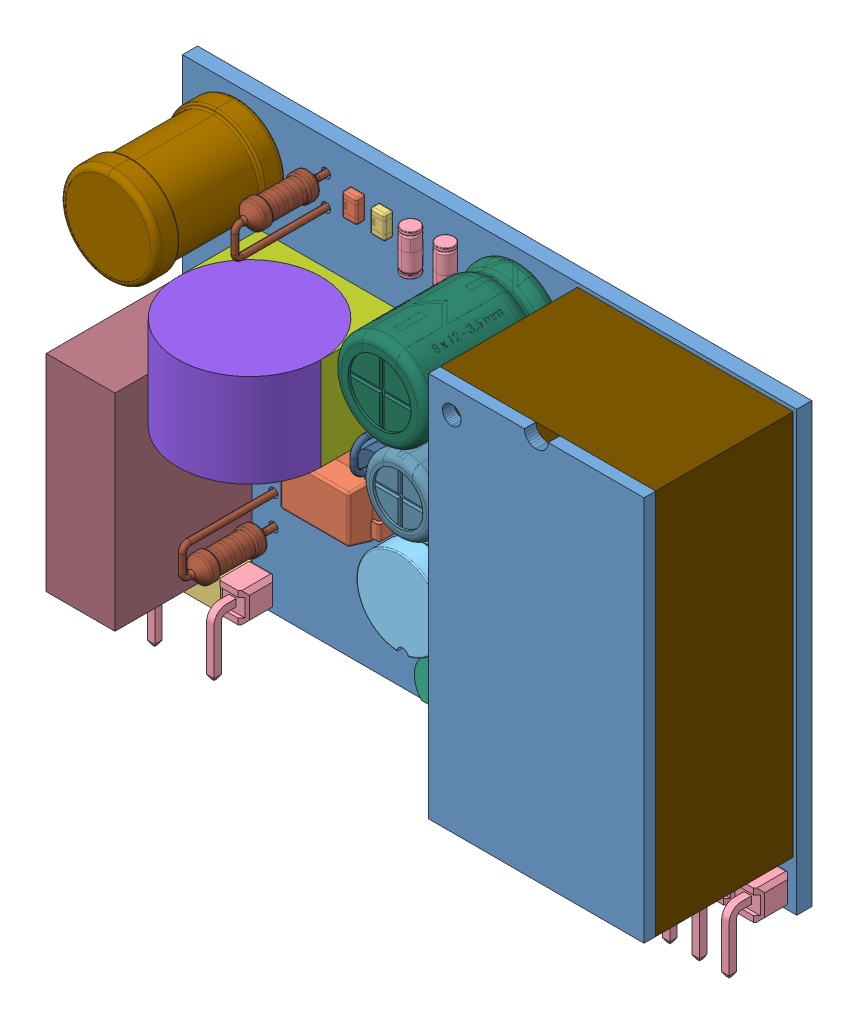
SolidWorks assembly KQ-130F, configuration Default. Lengths in mm.
Overall size (52.7 40.92 18.15).
108 component instances, 25 part files, 0 mates.
Components (placement in the parent):
- KQ-130F.step-1: KQ-130F.step [Default] at origin size (52.7 40.92 18.15)
  - Board.step-1: Board.step [Default] at origin size (52.7 37.6 1.29)
    - Open CASCADE STEP translator 6.8 4.1.1.step-1: Open CASCADE STEP translator 6.8 4.1.1.step [Default] at (0 0 -1.2914) size (52.7 37.6 1.29)
  - Designator39.step-1: Designator39.step [Default] at origin size (1.25 2 0.78)
    - User_Library-0805_SMD_Resistor.step-1: User_Library-0805_SMD_Resistor.step [Default] at (77.385 48.11 0) x (0 1 0) z (1 0 0) size (2 0.78 1.25)
  - Designator38.step-1: Designator38.step [Default] at origin size (1.25 2 0.78)
    - SW3dPS-0805_SMD_Capacitor.step-1: SW3dPS-0805_SMD_Capacitor.step [Default] at (77.345 42.3 0) x (0 1 0) z (1 0 0) size (2 0.78 1.25)
  - Designator37.step-1: Designator37.step [Default] at origin size (1.25 2 0.78)
    - User_Library-0805_SMD_Resistor.step-1: User_Library-0805_SMD_Resistor.step [Default] at (67.215 44.89 0) x (0 -1 0) z (-1 0 0) size (2 0.78 1.25)
  - Designator36.step-1: Designator36.step [Default] at origin size (1.51 3.5 1.51)
    - User_Library-Diode_MELF.step-1: User_Library-Diode_MELF.step [Default] at (63.8201 43.3999 0.75) x (0 1 0) z (0 0 1) size (3.5 1.51 1.51)
  - Designator35.step-1: Designator35.step [Default] at origin size (3.5 1.51 1.51)
    - User_Library-Diode_MELF.step-1: User_Library-Diode_MELF.step [Default] at (54.6999 53.3999 0.75) x (1 0 0) z (0 0 1) size (3.5 1.51 1.51)
  - Designator34.step-1: Designator34.step [Default] at origin size (1.51 3.5 1.51)
    - User_Library-Diode_MELF.step-1: User_Library-Diode_MELF.step [Default] at (65.2999 68.7001 0.75) x (0 -1 0) z (0 0 1) size (3.5 1.51 1.51)
  - Designator33.step-1: Designator33.step [Default] at origin size (1.25 2 0.78)
    - SW3dPS-0805_SMD_Capacitor.step-1: SW3dPS-0805_SMD_Capacitor.step [Default] at (62.485 69.1 0) x (0 1 0) z (1 0 0) size (2 0.78 1.25)
  - Designator32.step-1: Designator32.step [Default] at origin size (1.51 3.5 1.51)
    - User_Library-Diode_MELF.step-1: User_Library-Diode_MELF.step [Default] at (68.3001 68.9999 0.75) x (0 1 0) z (0 0 1) size (3.5 1.51 1.51)
  - Designator31.step-1: Designator31.step [Default] at origin size (1.25 2 0.78)
    - User_Library-0805_SMD_Resistor.step-1: User_Library-0805_SMD_Resistor.step [Default] at (60.085 69.11 0) x (0 1 0) z (1 0 0) size (2 0.78 1.25)
  - Designator30.step-1: Designator30.step [Default] at origin size (1.6 3.2 1)
    - User_Library-1206_SMD_Capacitor.step-1: User_Library-1206_SMD_Capacitor.step [Default] at (69.9999 60 0) x (0 1 0) z (1 0 0) size (3.2 1 1.6)
  - Designator17.step-1: Designator17.step [Default] at origin size (5.58 3.97 7.7)
    - TO-92-1.step-1: TO-92-1.step [Default] at (72.6601 41.8789 0.7086) x (1 0 0) z (0 0 1) size (5.58 3.97 7.7)
  - Designator16.step-1: Designator16.step [Default] at origin size (12.3 8 13.15)
    - 5896934704.step-1: 5896934704.step [Default] at (57.75 58.9 0) size (12.3 8 7)
      - Extruded.step-1: Extruded.step [Default] at origin size (12.3 8 7)
    - 5896934224.step-1: 5896934224.step [Default] at (57.75 62.9 7) x (1 0 0) z (0 -1 0) size (12.3 12.3 8)
      - Cylinder.step-1: Cylinder.step [Default] at origin size (12.3 12.3 8)
  - Designator14.step-1: Designator14.step [Default] at origin size (8.3 8.3 16.2)
    - SW3dPS-CT187LY-271.step-1: SW3dPS-CT187LY-271.step [Default] at (49.81 67.8001 0) x (1 0 0) z (0 -1 0) size (8.3 16.2 8.3)
  - Designator15.step-1: Designator15.step [Default] at origin size (2.5 4.04 9.55)
    - Diode.step-1: Diode.step [Default] at (66.1999 55 0.2) x (-1 0 0) z (0 0 1) size (2.5 4.04 9.55)
  - Designator14-1.step-1: Designator14-1.step [Default] at origin size (2.2 3.89 11.06)
    - Widerstand.step-1: Widerstand.step [Default] at (57.3001 69.9501 4) size (2.2 3.89 11.06)
  - Designator13.step-1: Designator13.step [Default] at origin size (5.9 17.7 15.25)
    - 5896932864.step-1: 5896932864.step [Default] at (48 40.6 -3.5) size (0.6 0.6 3.5)
      - Extruded-0.step-1: Extruded-0.step [Default] at origin size (0.6 0.6 3.5)
    - 5896932864.step-2: 5896932864.step [Default] at (48 54.3002 -3.5) size (0.6 0.6 3.5)
      - Extruded-0.step-1: Extruded-0.step [Default] at origin size (0.6 0.6 3.5)
    - 5896933104.step-1: 5896933104.step [Default] at (48.0001 47.45 0) size (5.9 17.7 11.75)
      - Extruded-1.step-1: Extruded-1.step [Default] at origin size (5.9 17.7 11.75)
  - Designator12.step-1: Designator12.step [Default] at origin size (6.3 6.44 14.21)
    - User_Library-Cap-EL(6_3x11-2_5).step-1: User_Library-Cap-EL(6_3x11-2_5).step [Default] at (74.9688 60.3385 0.5) x (0 1 0) z (0 0 1) size (6.44 6.3 14.21)
  - Designator11.step-1: Designator11.step [Default] at origin size (8 8.15 15.6)
    - User_Library-Cap-EL(8x12-3_5)T.step-1: User_Library-Cap-EL(8x12-3_5)T.step [Default] at (74.1999 68.2001 0) x (0 1 0) z (0 0 1) size (8.15 8 15.6)
  - Open CASCADE STEP translator 6.8 4.20.step-1: Open CASCADE STEP translator 6.8 4.20.step [Default] at origin size (18.5 33.1 15.26)
    - 1P.step-1: 1P.step [Default] at (80.9001 45.5599 -7.21) x (0 -1 0) z (-1 0 0) size (2.54 11 2.54)
      - pin.step-1: pin.step [Default] at (0 4.751 0) size (0.66 11 0.66)
      - plastic.step-1: plastic.step [Default] at (0 7.751 0) size (2.54 2.5 2.54)
    - 1P.step-2: 1P.step [Default] at (80.9001 48.0999 -7.21) x (0 -1 0) z (-1 0 0) size (2.54 11 2.54)
      - pin.step-1: pin.step [Default] at (0 4.751 0) size (0.66 11 0.66)
      - plastic.step-1: plastic.step [Default] at (0 7.751 0) size (2.54 2.5 2.54)
    - 1P.step-3: 1P.step [Default] at (80.9001 55.7199 -7.21) x (0 -1 0) z (-1 0 0) size (2.54 11 2.54)
      - pin.step-1: pin.step [Default] at (0 4.751 0) size (0.66 11 0.66)
      - plastic.step-1: plastic.step [Default] at (0 7.751 0) size (2.54 2.5 2.54)
    - 1P.step-4: 1P.step [Default] at (80.9001 58.2599 -7.21) x (0 -1 0) z (-1 0 0) size (2.54 11 2.54)
      - pin.step-1: pin.step [Default] at (0 4.751 0) size (0.66 11 0.66)
      - plastic.step-1: plastic.step [Default] at (0 7.751 0) size (2.54 2.5 2.54)
    - 1P.step-5: 1P.step [Default] at (80.9001 50.6399 -7.21) x (0 -1 0) z (-1 0 0) size (2.54 11 2.54)
      - pin.step-1: pin.step [Default] at (0 4.751 0) size (0.66 11 0.66)
      - plastic.step-1: plastic.step [Default] at (0 7.751 0) size (2.54 2.5 2.54)
    - 1P.step-6: 1P.step [Default] at (80.9001 53.1799 -7.21) x (0 -1 0) z (-1 0 0) size (2.54 11 2.54)
      - pin.step-1: pin.step [Default] at (0 4.751 0) size (0.66 11 0.66)
      - plastic.step-1: plastic.step [Default] at (0 7.751 0) size (2.54 2.5 2.54)
    - 1P.step-7: 1P.step [Default] at (80.9001 65.8799 -7.21) x (0 -1 0) z (-1 0 0) size (2.54 11 2.54)
      - pin.step-1: pin.step [Default] at (0 4.751 0) size (0.66 11 0.66)
      - plastic.step-1: plastic.step [Default] at (0 7.751 0) size (2.54 2.5 2.54)
    - 1P.step-8: 1P.step [Default] at (80.9001 68.4199 -7.21) x (0 -1 0) z (-1 0 0) size (2.54 11 2.54)
      - pin.step-1: pin.step [Default] at (0 4.751 0) size (0.66 11 0.66)
      - plastic.step-1: plastic.step [Default] at (0 7.751 0) size (2.54 2.5 2.54)
    - 1P.step-9: 1P.step [Default] at (80.9001 60.7999 -7.21) x (0 -1 0) z (-1 0 0) size (2.54 11 2.54)
      - pin.step-1: pin.step [Default] at (0 4.751 0) size (0.66 11 0.66)
      - plastic.step-1: plastic.step [Default] at (0 7.751 0) size (2.54 2.5 2.54)
    - 1P.step-10: 1P.step [Default] at (80.9001 63.3399 -7.21) x (0 -1 0) z (-1 0 0) size (2.54 11 2.54)
      - pin.step-1: pin.step [Default] at (0 4.751 0) size (0.66 11 0.66)
      - plastic.step-1: plastic.step [Default] at (0 7.751 0) size (2.54 2.5 2.54)
    - 1P.step-11: 1P.step [Default] at (80.9001 43.0199 -7.21) x (0 -1 0) z (-1 0 0) size (2.54 11 2.54)
      - pin.step-1: pin.step [Default] at (0 4.751 0) size (0.66 11 0.66)
      - plastic.step-1: plastic.step [Default] at (0 7.751 0) size (2.54 2.5 2.54)
    - 5896931904.step-1: 5896931904.step [Default] at (88.15 55.72 0) size (18.5 33.1 11.8)
      - Extruded-2.step-1: Extruded-2.step [Default] at origin size (18.5 33.1 11.8)
    - 5896929504.step-1: 5896929504.step [Default] at (88.15 55.72 11.8) size (18.5 33.1 1)
  - Designator9.step-1: Designator9.step [Default] at origin size (7.87 4.6 6.31)
    - User_Library-DIP4.step-1: User_Library-DIP4.step [Default] at (60.0609 48.8299 2) x (1 0 0) z (0 0 1) size (7.87 4.6 6.31)
  - Designator7.step-1: Designator7.step [Default] at origin size (2.2 3.89 11.06)
    - Widerstand.step-1: Widerstand.step [Default] at (52.7999 41.3999 4) x (-1 0 0) z (0 0 1) size (2.2 3.89 11.06)
  - Designator6.step-1: Designator6.step [Default] at origin size (4.04 2.5 9.55)
    - Diode.step-1: Diode.step [Default] at (76.7999 55.1999 0.2) x (0 -1 0) z (0 0 1) size (2.5 4.04 9.55)
  - Designator5.step-1: Designator5.step [Default] at origin size (7.63 6.29 6.17)
    - 6243679216.step-1: 6243679216.step [Default] at (49.2825 36.698 0) size (3.33 2.55 2.7)
      - Extruded-3.step-1: Extruded-3.step [Default] at origin size (3.33 2.55 2.7)
    - Pin_Header_1x1_TH_Angle_Pitch_2.54mm.step-1: Pin_Header_1x1_TH_Angle_Pitch_2.54mm.step [Default] at (56.8927 34.881 4.12) x (-1 0 0) z (0 1 0) size (2.55 6.17 6.29)
    - Pin_Header_1x1_TH_Angle_Pitch_2.54mm.step-2: Pin_Header_1x1_TH_Angle_Pitch_2.54mm.step [Default] at (51.8127 34.881 4.12) x (-1 0 0) z (0 1 0) size (2.55 6.17 6.29)
  - Designator3.step-1: Designator3.step [Default] at origin size (17.79 6.29 6.19)
    - Pin_Header_1x1_TH_Angle_Pitch_2.54mm.step-1: Pin_Header_1x1_TH_Angle_Pitch_2.54mm.step [Default] at (88.3892 34.88 4.1) x (-1 0 0) z (0 1 0) size (2.55 6.17 6.29)
    - Pin_Header_1x1_TH_Angle_Pitch_2.54mm.step-2: Pin_Header_1x1_TH_Angle_Pitch_2.54mm.step [Default] at (85.8492 34.88 4.1) x (-1 0 0) z (0 1 0) size (2.55 6.17 6.29)
    - Pin_Header_1x1_TH_Angle_Pitch_2.54mm.step-3: Pin_Header_1x1_TH_Angle_Pitch_2.54mm.step [Default] at (90.9327 34.881 4.12) x (-1 0 0) z (0 1 0) size (2.55 6.17 6.29)
    - Pin_Header_1x1_TH_Angle_Pitch_2.54mm.step-4: Pin_Header_1x1_TH_Angle_Pitch_2.54mm.step [Default] at (93.4727 34.881 4.12) x (-1 0 0) z (0 1 0) size (2.55 6.17 6.29)
    - Pin_Header_1x1_TH_Angle_Pitch_2.54mm.step-5: Pin_Header_1x1_TH_Angle_Pitch_2.54mm.step [Default] at (96.0127 34.881 4.12) x (-1 0 0) z (0 1 0) size (2.55 6.17 6.29)
    - Pin_Header_1x1_TH_Angle_Pitch_2.54mm.step-6: Pin_Header_1x1_TH_Angle_Pitch_2.54mm.step [Default] at (101.0927 34.881 4.12) x (-1 0 0) z (0 1 0) size (2.55 6.17 6.29)
    - Pin_Header_1x1_TH_Angle_Pitch_2.54mm.step-7: Pin_Header_1x1_TH_Angle_Pitch_2.54mm.step [Default] at (98.5527 34.881 4.12) x (-1 0 0) z (0 1 0) size (2.55 6.17 6.29)
  - Free-Models.step-1: Free-Models.step [Default] at origin size (8.02 7.89 11)
    - STEP_inductor_PCB_(assembly).step-1: STEP_inductor_PCB_(assembly).step [Default] at (-104.7161 48.9768 8) x (1 0 0) z (0 -1 0) size (8.02 11 7.89)
      - inductor_PCB_(BODY+PINS).step-1: inductor_PCB_(BODY+PINS).step [Default] at (176.9711 0.6423 -0.8154) x (0.997306 0 -0.073354) z (-0.073354 0 -0.997306) size (7.37 11 7.37)
      - inductor_PCB_(WIRE1).step-1: inductor_PCB_(WIRE1).step [Default] at (176.9739 -1.4582 -0.844) x (1 0 0) z (0 -1 0) size (5.4 6.61 6.17)
      - inductor_PCB_(WIRE2).step-1: inductor_PCB_(WIRE2).step [Default] at (176.9752 -4.9372 -0.8366) x (0.087156 0 0.996195) z (0 1 0) size (5.01 6.35 6.76)
